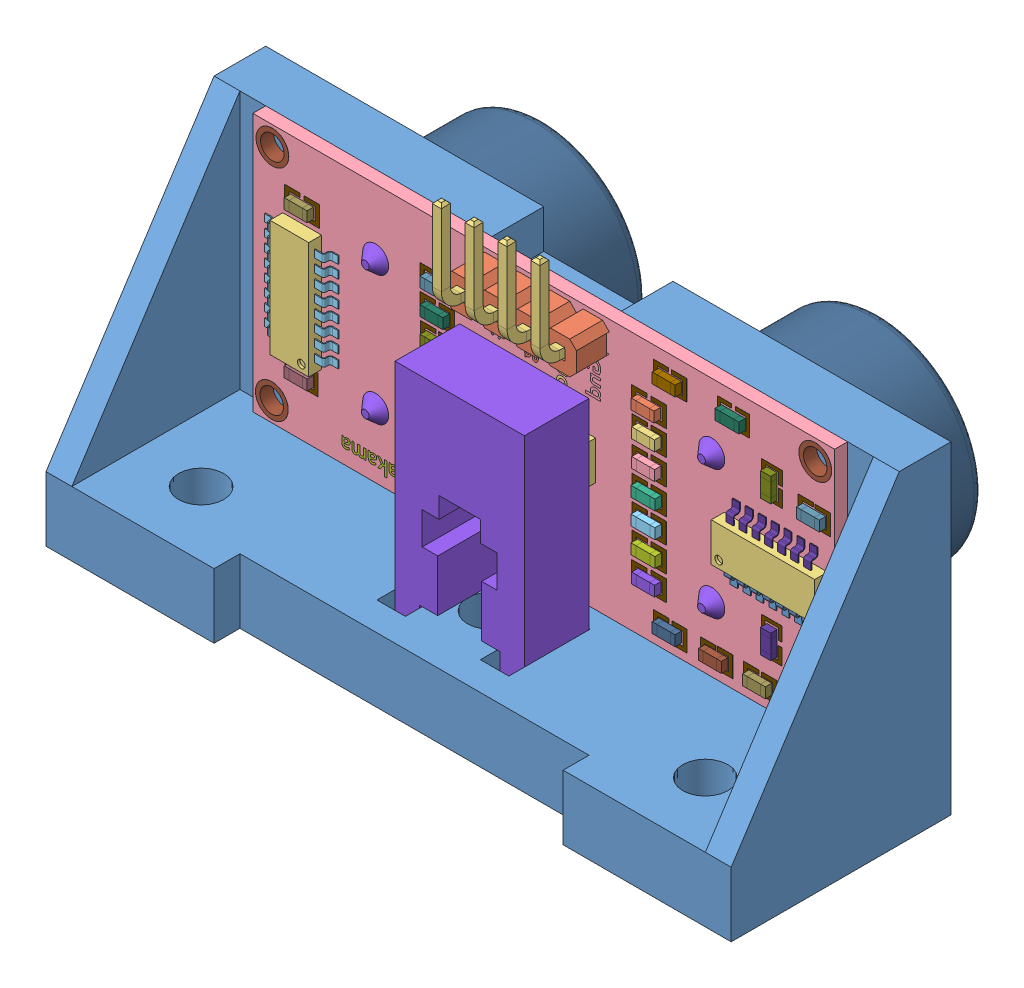
SolidWorks assembly cummatsieuamdon, configuration Default. Lengths in mm.
Overall size (53 30.57 25).
63 component instances, 62 part files, 6 mates.
Components (placement in the parent):
- ga lap ultrasonic v5-1: ga lap ultrasonic v5 [Default] at (-305.8263 5.4763 137.5129) size (53 25 17)
- 6. HC-04HC-04.stp-1: 6. HC-04HC-04.stp [Default] at (-291.7459 14.1831 142.5129) x (1 0 0) z (0 0 -1) size (45 25.57 17.46)
  - HC-04Array.stp-1: HC-04Array.stp [Default] at origin size (10.16 2.54 2.54)
  - HC-04Array001.stp-1: HC-04Array001.stp [Default] at (0 0 1) size (8.32 7.52 6.46)
  - HC-04Placa.stp-1: HC-04Placa.stp [Default] at origin size (45 20 1)
  - HC-04Pad003.stp-1: HC-04Pad003.stp [Default] at (0 0 1) size (10.52 3.38 0.2)
  - HC-04Fillet.stp-1: HC-04Fillet.stp [Default] at (0 0 1) size (10.1 2.84 3)
  - HC-04Array002.stp-1: HC-04Array002.stp [Default] at origin size (9.62 2 1)
  - HC-04Array003.stp-1: HC-04Array003.stp [Default] at (0 0 1) size (28 12 0.8)
  - HC-04Fusion.stp-1: HC-04Fusion.stp [Default] at origin size (6 2 1)
  - HC-04Fillet001.stp-1: HC-04Fillet001.stp [Default] at (0 0 1) size (42 16 12)
  - HC-04Pad005.stp-1: HC-04Pad005.stp [Default] at (0 0 1) size (39.16 13 0.2)
  - HC-04Pad006.stp-1: HC-04Pad006.stp [Default] at (0 0 1) size (35.01 9.04 7)
  - HC-04Fusion001.stp-1: HC-04Fusion001.stp [Default] at (0 0 8) size (31 5 1.5)
  - HC-04Clone_of_Fusion002.stp-1: HC-04Clone_of_Fusion002.stp [Default] at (47.2 -5.5 12.6) size (13 13 0.15)
  - HC-04Clone_of_Fusion003.stp-1: HC-04Clone_of_Fusion003.stp [Default] at (21.2 -5.5 12.6) size (13 13 0.15)
  - HC-04Array005.stp-1: HC-04Array005.stp [Default] at origin size (9.62 2 1)
  - HC-04Array002002.stp-1: HC-04Array002002.stp [Default] at (-5.9 0.1 0.15) size (6.57 1.4 0.56)
  - HC-04Clone_of_Array002002.stp-1: HC-04Clone_of_Array002002.stp [Default] at (-23.9 0.1 0.15) size (6.57 1.4 0.56)
  - HC-04Array002003.stp-1: HC-04Array002003.stp [Default] at (-6.05 0 0.15) size (6.57 1.4 0.56)
  - HC-04Clone_of_Array002003.stp-1: HC-04Clone_of_Array002003.stp [Default] at (-24.05 0 0.15) size (6.57 1.4 0.56)
  - HC-04Integrados.stp-1: HC-04Integrados.stp [Default] at origin size (42.14 9 1)
  - HC-04ShapeString.stp-1: HC-04ShapeString.stp [Default] at (-3.2 -7 1.01) x (0 1 0) z (0 0 1) size (2.53 1.13 0.01)
  - HC-04ShapeString001.stp-1: HC-04ShapeString001.stp [Default] at (-0.6 -7 1.01) x (0 1 0) z (0 0 1) size (2.66 1.45 0.01)
  - HC-04ShapeString002.stp-1: HC-04ShapeString002.stp [Default] at (1.9 -7 1.01) x (0 1 0) z (0 0 1) size (3.21 1.16 0.01)
  - HC-04ShapeString003.stp-1: HC-04ShapeString003.stp [Default] at (4.5 -7 1.01) x (0 1 0) z (0 0 1) size (2.71 1.16 0.01)
  - HC-04ShapeString004.stp-1: HC-04ShapeString004.stp [Default] at (-19.5 -9.3 1.01) size (1.84 2.34 0.01)
  - HC-04ShapeString005.stp-1: HC-04ShapeString005.stp [Default] at (17.5 -9.3 1.01) size (1.82 2.34 0.01)
  - HC-04ShapeString006.stp-1: HC-04ShapeString006.stp [Default] at (-3 3.7 1.01) size (5.52 1.41 0.01)
  - HC-04Pad008.stp-1: HC-04Pad008.stp [Default] at (0 0 -0.01) size (44.56 19.6 1.02)
  - HC-04Scale004.stp-1: HC-04Scale004.stp [Default] at (-1.9 -21.5 -1.5) x (0 1 0) z (0 0 1) size (0.8 1.77 0.5)
  - HC-04Scale027.stp-1: HC-04Scale027.stp [Default] at (-1.9 -10.2323 -1.5) x (0 1 0) z (0 0 1) size (0.8 1.77 0.5)
  - HC-04Scale028.stp-1: HC-04Scale028.stp [Default] at (8.5984 -21.5 -1.5) x (0 1 0) z (0 0 1) size (0.8 1.77 0.5)
  - HC-04Scale029.stp-1: HC-04Scale029.stp [Default] at (8.5984 -19.5867 -1.5) x (0 1 0) z (0 0 1) size (0.8 1.77 0.5)
  - HC-04Scale030.stp-1: HC-04Scale030.stp [Default] at (8.5984 -17.5982 -1.5) x (0 1 0) z (0 0 1) size (0.8 1.77 0.5)
  - HC-04Scale031.stp-1: HC-04Scale031.stp [Default] at (8.5984 -15.6427 -1.5) x (0 1 0) z (0 0 1) size (0.8 1.77 0.5)
  - HC-04Scale032.stp-1: HC-04Scale032.stp [Default] at (8.5984 -11.6848 -1.5) x (0 1 0) z (0 0 1) size (0.8 1.77 0.5)
  - HC-04Scale033.stp-1: HC-04Scale033.stp [Default] at (-26.74 -2 -1.5) x (0 1 0) z (0 0 1) size (0.8 1.85 0.5)
  - HC-04Scale034.stp-1: HC-04Scale034.stp [Default] at (24.9371 -21.5 -1.5) x (0 1 0) z (0 0 1) size (0.8 1.77 0.5)
  - HC-04Scale035.stp-1: HC-04Scale035.stp [Default] at (24.9691 -19.5867 -1.5) x (0 1 0) z (0 0 1) size (0.8 1.77 0.5)
  - HC-04Scale036.stp-1: HC-04Scale036.stp [Default] at (24.9742 -17.5982 -1.5) x (0 1 0) z (0 0 1) size (0.8 1.77 0.5)
  - HC-04Scale037.stp-1: HC-04Scale037.stp [Default] at (-10.4013 -2 -1.5) x (0 1 0) z (0 0 1) size (0.8 1.85 0.5)
  - HC-04Scale038.stp-1: HC-04Scale038.stp [Default] at (-10.4013 -3.9266 -1.5) x (0 1 0) z (0 0 1) size (0.8 1.85 0.5)
  - HC-04Scale039.stp-1: HC-04Scale039.stp [Default] at (-10.4013 -0.0734 -1.5) x (0 1 0) z (0 0 1) size (0.8 1.85 0.5)
  - HC-04Scale040.stp-1: HC-04Scale040.stp [Default] at (24.9742 -9.855 -1.5) x (0 1 0) z (0 0 1) size (0.8 1.77 0.5)
  - HC-04Scale041.stp-1: HC-04Scale041.stp [Default] at (26.5673 -24.0564 -1.5) x (0 1 0) z (0 0 1) size (0.8 1.77 0.5)
  - HC-04Scale042.stp-1: HC-04Scale042.stp [Default] at (26.5673 -7.3333 -1.5) x (0 1 0) z (0 0 1) size (0.8 1.77 0.5)
  - HC-04Scale043.stp-1: HC-04Scale043.stp [Default] at (30.1435 -7.3333 -1.5) x (0 1 0) z (0 0 1) size (0.8 1.77 0.5)
  - HC-04Scale044.stp-1: HC-04Scale044.stp [Default] at (33.5459 -7.3333 -1.5) x (0 1 0) z (0 0 1) size (0.8 1.77 0.5)
  - HC-04Scale045.stp-1: HC-04Scale045.stp [Default] at (37.7181 -11.1827 -1.5) x (0 1 0) z (0 0 1) size (0.8 1.77 0.5)
  - HC-04Scale046.stp-1: HC-04Scale046.stp [Default] at (37.7181 -20.5932 -1.5) x (0 1 0) z (0 0 1) size (0.8 1.77 0.5)
  - HC-04Scale047.stp-1: HC-04Scale047.stp [Default] at (-3.9042 -12.3288 -1.5) x (0 1 0) z (0 0 1) size (0.8 1.85 0.5)
  - HC-04Scale048.stp-1: HC-04Scale048.stp [Default] at (13.5402 13.2894 -1.5) size (0.8 1.85 0.5)
  - HC-04Scale049.stp-1: HC-04Scale049.stp [Default] at (13.5402 23.7909 -1.5) size (0.8 1.85 0.5)
  - HC-04Pad009.stp-1: HC-04Pad009.stp [Default] x (1 0 0) z (0 0 -1) size (42.21 18.43 0.01)
  - HC-04ShapeString007.stp-1: HC-04ShapeString007.stp [Default] at (-3.2 -7 -0.1) x (0 1 0) z (0 0 1) size (2.53 1.13 0.01)
  - HC-04ShapeString008.stp-1: HC-04ShapeString008.stp [Default] at (-0.6 -7 -0.1) x (0 1 0) z (0 0 1) size (2.66 1.45 0.01)
  - HC-04ShapeString009.stp-1: HC-04ShapeString009.stp [Default] at (1.9 -7 -0.1) x (0 1 0) z (0 0 1) size (3.21 1.16 0.01)
  - HC-04ShapeString010.stp-1: HC-04ShapeString010.stp [Default] at (4.5 -7 -0.1) x (0 1 0) z (0 0 1) size (2.71 1.16 0.01)
  - HC-04Fusion002.stp-1: HC-04Fusion002.stp [Default] at origin size (5.7 7.57 0.56)
  - HC-04ShapeString011.stp-1: HC-04ShapeString011.stp [Default] at (-17.5 8.4 1.1) size (7.91 1.16 0.01)
  - HC-04ShapeString012.stp-1: HC-04ShapeString012.stp [Default] at (-7.5 8 -0.1) x (-1 0 0) z (0 0 -1) size (7.91 1.16 0.01)
- 12.ganh-1: 12.ganh [Default] at (-291.7459 10.0832 144.0129) x (1 0 0) z (0 -1 0) size (10 5 19)
Mates (geometry in assembly coordinates):
- Coincident1: coincident anti-aligned: plane of ga lap ultrasonic v5-1 through (-305.8263 5.4763 141.5129) normal (0 0 1); plane of 6. HC-04HC-04.stp-1/HC-04Placa.stp-1 through (-314.2459 4.1831 141.5129) normal (0 0 -1)
- Concentric1: concentric anti-aligned: cylinder of ga lap ultrasonic v5-1 through (-304.7459 14.1832 141.5129) axis (0 0 -1) radius 8.5; cylinder of 6. HC-04HC-04.stp-1/HC-04Fillet001.stp-1 through (-304.7459 14.1832 141.5129) axis (0 0 1) radius 8
- Concentric2: concentric anti-aligned: cylinder of ga lap ultrasonic v5-1 through (-278.7459 14.1832 141.5129) axis (0 0 -1) radius 8.5; cylinder of 6. HC-04HC-04.stp-1/HC-04Fillet001.stp-1 through (-278.7459 14.1832 141.5129) axis (0 0 1) radius 8
- Coincident2: coincident anti-aligned: plane of ga lap ultrasonic v5-1 through (-291.7459 4.1832 154.5129) normal (0 1 0); plane of 12.ganh-1 through (-291.7459 4.1832 149.0129) normal (0 -1 0)
- Width1: width aligned: plane of ga lap ultrasonic v5-1 through (-296.8459 0.6832 144.0129) normal (1 0 0); plane of ga lap ultrasonic v5-1 through (-286.6459 0.6832 144.0129) normal (-1 0 0); plane of 12.ganh-1 through (-286.7459 10.0832 149.0129) normal (1 0 0); plane of 12.ganh-1 through (-296.7459 10.0832 149.0129) normal (-1 0 0)
- Coincident4: coincident anti-aligned: plane of ga lap ultrasonic v5-1 through (-296.8459 0.6832 144.0129) normal (0 0 1); plane of 12.ganh-1 through (-291.7459 10.0832 144.0129) normal (0 0 -1)
